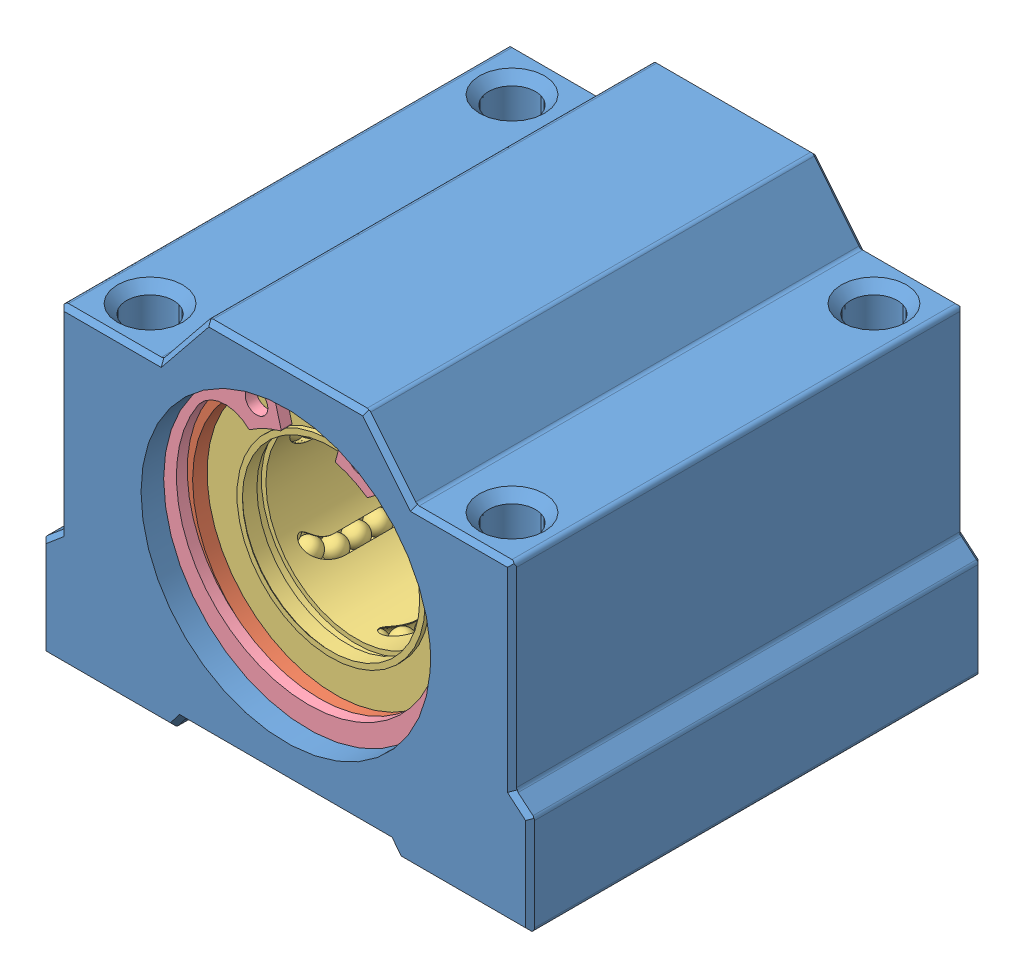
SolidWorks assembly SMA20, configuration Default. Lengths in mm.
Overall size (54 41 50).
6 component instances, 4 part files, 8 mates.
Components (placement in the parent):
- SMA20-1-1: SMA20-1 [Default] at (0.4328 26.8313 -29.5298) size (54 41 50)
- LM20-1: LM20 [Default] at (2.579 6.0628 -5.1402) size (32 32 42)
  - LM20-1-1: LM20-1 [Default] at (-2.1463 0.7685 -20.3896) size (32 32 42)
  - LM20-2-1: LM20-2 [Default] at (-16.3463 0.7685 20.6104) x (0 0 -1) z (1 0 0) size (40 28.4 28.4)
- circlip for bores normal_din-1: circlip for bores normal_din [Circlip DIN 472 - 32 x 1.2] at (0.4328 6.8313 -25.8298) x (-0.999999 0.001088 0) z (0 0 1) size (33.7 33.12 1.2)
- circlip for bores normal_din-4: circlip for bores normal_din [Circlip DIN 472 - 32 x 1.2] at (0.4328 6.8313 17.9702) x (-0.999999 -0.001088 0) z (0 0 1) size (33.7 33.12 1.2)
Mates (geometry in assembly coordinates):
- Concentric1: concentric aligned: cylinder of SMA20-1-1 through (0.4328 6.8313 20.4702) axis (0 0 -1) radius 16; cylinder of LM20-1/LM20-1-1 through (0.4328 6.8313 16.4702) axis (0 0 -1) radius 16
- Distance1: distance = 4 mm aligned: plane of LM20-1/LM20-1-1 through (0.4328 6.8313 16.4702) normal (0 0 1); plane of SMA20-1-1 through (-26.5672 -14.1687 20.4702) normal (0 0 1)
- Concentric2: concentric anti-aligned: cylinder of SMA20-1-1 through (0.4328 6.8313 -29.5298) axis (0 0 -1) radius 17; cylinder of circlip for bores normal_din-1 through (0.4328 6.8313 -27.0298) axis (0 0 1) radius 16.85
- Concentric4: concentric anti-aligned: cylinder of SMA20-1-1 through (0.4328 6.8313 20.4702) axis (0 0 -1) radius 16; cylinder of circlip for bores normal_din-4 through (0.4328 6.8313 16.7702) axis (0 0 1) radius 16.85
- Coincident4: coincident anti-aligned: plane of SMA20-1-1 through (0.4328 22.8313 17.9702) normal (0 0 -1); plane of circlip for bores normal_din-4 through (0.4328 6.8313 17.9702) normal (0 0 1)
- Coincident6: coincident aligned: circle of SMA20-1-1; plane of circlip for bores normal_din-1 through (0.4328 6.8313 -27.0298) normal (0 0 -1)
- Angle1: planar angle = 1.308997 rad aligned: plane of circlip for bores normal_din-4 through (4.7939 23.1072 16.7702) normal (-0.965926 0.258819 0); plane of SMA20-1-1 through (9.1828 26.8313 20.4702) normal (0 1 0)
- Angle2: planar angle = 1.308997 rad aligned: plane of circlip for bores normal_din-1 through (-3.9283 23.1072 -27.0298) normal (0.965926 0.258819 0); plane of SMA20-1-1 through (9.1828 26.8313 20.4702) normal (0 1 0)
